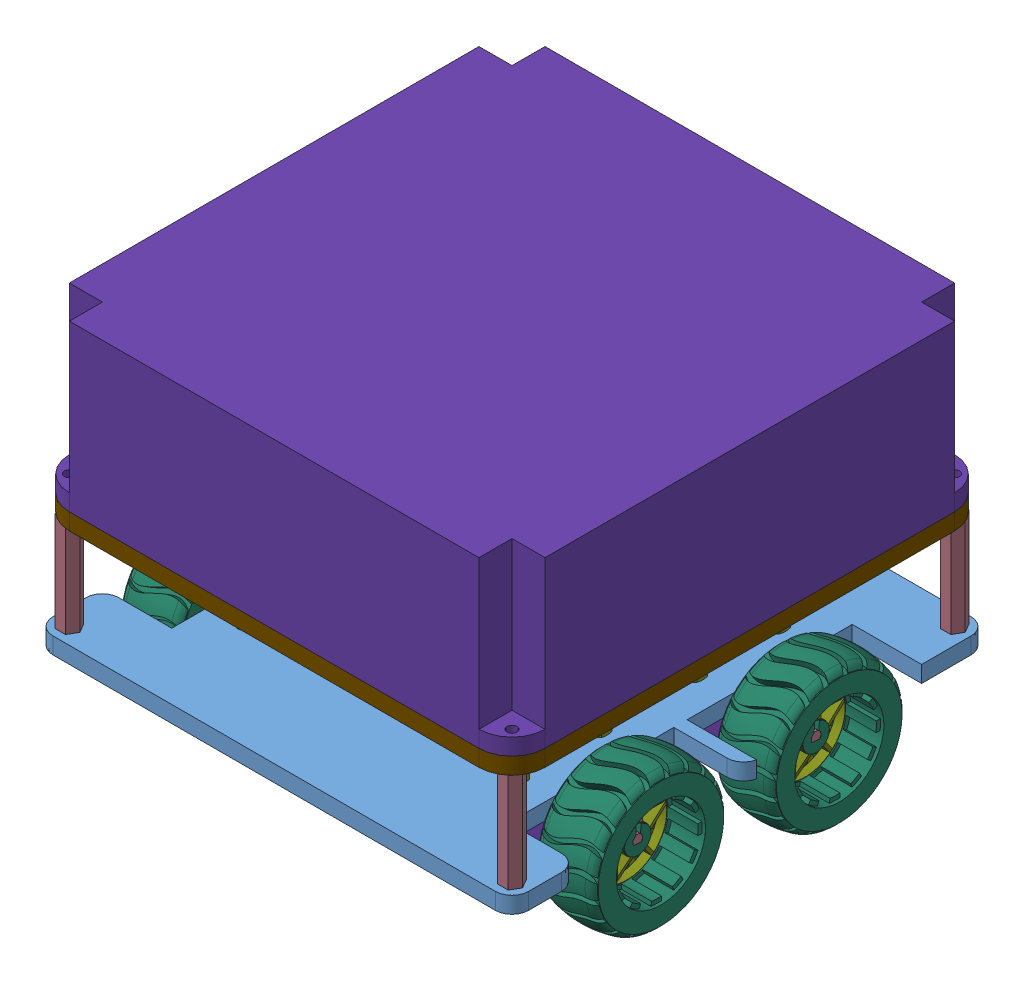
SolidWorks assembly 4 WHEELED BOT, configuration Default. Lengths in mm.
Overall size (144.48 119.43 144).
160 component instances, 35 part files, 86 mates.
Components (placement in the parent):
- BASE-1: BASE [Default] at (33.0776 85.5576 114.3688) size (144 5 144)
- Motor complete assembly-1: Motor complete assembly [Default] at (60.6046 55.5446 163.4077) x (1 0 0) z (0 1 0) size (47.72 49.6 49.13)
  - MOTOR ASSEMBLY-1: MOTOR ASSEMBLY [По умолчанию] at (3.7017 9.4456 12.6365) size (40.48 13.3 19.35)
    - H-1: H [По умолчанию] at (2.1713 12.5934 12.3765) size (17.5 12.02 10)
    - spur gear_iso-1: spur gear_iso [ISO - Spur gear 0.25M 11T 20PA 1.5FW ---S11A75H50L1.0N] at (15.9213 12.5934 12.3765) x (1 0 0) z (0 0.090891 -0.995861) size (1.5 3.2 3.23)
    - I-1: I [По умолчанию] at (14.6713 12.5934 12.3765) x (0 1 0) z (1 0 0) size (12 10 0.8)
    - G-1: G [По умолчанию] at (17.9713 16.1934 15.3765) x (0 0 1) z (0 -1 0) size (3 2.5 3)
    - G-2: G [По умолчанию] at (15.4713 8.9934 9.3765) x (0 1 0) z (0 0 -1) size (3 2.5 3)
    - J-1: J [По умолчанию] at (17.9713 12.5934 12.3765) x (0 -1 0) z (1 0 0) size (12 10 0.8)
    - A-1: A [По умолчанию] at (22.9713 16.1934 15.3765) x (0 -0.998437 -0.055897) z (0 0.055897 -0.998437) size (3 4.2 3)
    - A-2: A [По умолчанию] at (18.7713 8.9934 9.3765) x (0 0.267458 -0.96357) z (0 -0.96357 -0.267458) size (3 4.2 3)
    - C-1: C [По умолчанию] at (22.9713 12.5934 12.3765) x (0 1 0) z (1 0 0) size (12 10 1.8)
    - spur gear_iso-2: spur gear_iso [ISO - Spur gear 0.25M 20T 20PA 1,5FW ---S20B6H1,7L0.8N] at (17.9713 12.5934 12.3765) x (-1 0 0) z (0 0.996827 -0.079597) size (1.7 5.45 5.45)
    - F-1: F [По умолчанию] at (17.9713 9.3434 14.3765) x (0 0.378034 -0.925792) z (0 -0.925792 -0.378034) size (0.75 5.8 0.75)
    - E-1: E [По умолчанию] at (17.9713 12.5934 12.3765) x (0 0.298251 0.954488) z (0 0.954488 -0.298251) size (0.75 3.5 0.75)
    - spur gear_iso-3: spur gear_iso [ISO - Spur gear 0.25M 20T 20PA 1FW ---S20A75H50L0.8N] at (18.8713 12.5934 12.3765) x (1 0 0) z (0 0.821933 -0.569584) size (1 5.45 5.45)
    - spur gear_iso-4: spur gear_iso [ISO - Spur gear 0.25M 10T 20PA 1,3FW ---S10A75H50L0.8N] at (19.8713 12.5934 12.3765) x (1 0 0) z (0 -0.579316 0.815103) size (1.3 2.87 3)
    - spur gear_iso-6: spur gear_iso [ISO - Spur gear 0.25M 10T 20PA 1,7FW ---S10A75H50L0.8N] at (16.3713 9.3434 14.3765) x (1 0 0) z (0 -0.299679 -0.95404) size (1.7 2.87 3)
    - spur gear_iso-7: spur gear_iso [ISO - Spur gear 0.25M 20T 20PA 1,2FW ---S20A75H50L0.8N] at (19.9713 9.3434 14.3765) x (1 0 0) z (0 0.932152 0.362067) size (1.2 5.45 5.45)
    - D-1: D [По умолчанию] at (14.6713 15.8434 10.3765) x (0 0 -1) z (0 -1 0) size (0.75 9.1 0.75)
    - spur gear_iso-8: spur gear_iso [ISO - Spur gear 0.25M 20T 20PA 1,5FW ---S20A75H50L0.8N] at (15.9213 15.8434 10.3765) x (1 0 0) z (0 -0.974451 0.2246) size (1.5 5.45 5.45)
    - spur gear_iso-9: spur gear_iso [ISO - Spur gear 0.25M 10T 20PA 3,5FW ---S10A75H50L0.8N] at (17.4213 15.8434 10.3765) x (1 0 0) z (0 0.96714 0.254244) size (3.5 2.87 3)
    - motor back part-1: motor back part [Default] at (1.1713 12.5934 12.3765) x (0 0 1) z (-1 0 0) size (10 11.89 1.02)
    - B-2: B [По умолчанию] at (22.9713 12.5934 12.3765) x (0 0.071836 0.997416) z (0 0.997416 -0.071836) size (3 12.3 3)
    - K-2: K [Default] at (0.1713 12.5934 12.3765) x (0 -0.999909 0.013511) z (-1 0 0) size (12 19 7.88)
  - RC wheel-1: RC wheel [Default] at (14.1964 -16.5261 -2.5515) x (0 0.997416 -0.071836) z (1 0 0) size (46.42 45.91 18.48)
    - Housing-1: Housing [Default] at (36.5766 30.151 12.2766) size (46.42 45.91 18.48)
    - Hub-1: Hub [Default] at (36.5766 30.151 17.1766) x (-0.261271 -0.965266 0) z (-0.965266 0.261271 0) size (24.5 5.75 24.5)
  - gear motor clamp-1: gear motor clamp [Default] at (18.373 22.0389 30.013) x (0 1 0) z (-1 0 0) size (36 13 11)
- Motor complete assembly-2: Motor complete assembly [Default] at (60.6046 55.5446 109.4077) x (1 0 0) z (0 1 0) size (47.72 49.6 49.13)
  - MOTOR ASSEMBLY-1: MOTOR ASSEMBLY [По умолчанию] at (3.7017 9.4456 12.6365) size (40.48 13.3 19.35)
    - H-1: H [По умолчанию] at (2.1713 12.5934 12.3765) size (17.5 12.02 10)
    - spur gear_iso-1: spur gear_iso [ISO - Spur gear 0.25M 11T 20PA 1.5FW ---S11A75H50L1.0N] at (15.9213 12.5934 12.3765) x (1 0 0) z (0 0.090891 -0.995861) size (1.5 3.2 3.23)
    - I-1: I [По умолчанию] at (14.6713 12.5934 12.3765) x (0 1 0) z (1 0 0) size (12 10 0.8)
    - G-1: G [По умолчанию] at (17.9713 16.1934 15.3765) x (0 0 1) z (0 -1 0) size (3 2.5 3)
    - G-2: G [По умолчанию] at (15.4713 8.9934 9.3765) x (0 1 0) z (0 0 -1) size (3 2.5 3)
    - J-1: J [По умолчанию] at (17.9713 12.5934 12.3765) x (0 -1 0) z (1 0 0) size (12 10 0.8)
    - A-1: A [По умолчанию] at (22.9713 16.1934 15.3765) x (0 -0.998437 -0.055897) z (0 0.055897 -0.998437) size (3 4.2 3)
    - A-2: A [По умолчанию] at (18.7713 8.9934 9.3765) x (0 0.267458 -0.96357) z (0 -0.96357 -0.267458) size (3 4.2 3)
    - C-1: C [По умолчанию] at (22.9713 12.5934 12.3765) x (0 1 0) z (1 0 0) size (12 10 1.8)
    - spur gear_iso-2: spur gear_iso [ISO - Spur gear 0.25M 20T 20PA 1,5FW ---S20B6H1,7L0.8N] at (17.9713 12.5934 12.3765) x (-1 0 0) z (0 0.996827 -0.079597) size (1.7 5.45 5.45)
    - F-1: F [По умолчанию] at (17.9713 9.3434 14.3765) x (0 0.378034 -0.925792) z (0 -0.925792 -0.378034) size (0.75 5.8 0.75)
    - E-1: E [По умолчанию] at (17.9713 12.5934 12.3765) x (0 0.298251 0.954488) z (0 0.954488 -0.298251) size (0.75 3.5 0.75)
    - spur gear_iso-3: spur gear_iso [ISO - Spur gear 0.25M 20T 20PA 1FW ---S20A75H50L0.8N] at (18.8713 12.5934 12.3765) x (1 0 0) z (0 0.821933 -0.569584) size (1 5.45 5.45)
    - spur gear_iso-4: spur gear_iso [ISO - Spur gear 0.25M 10T 20PA 1,3FW ---S10A75H50L0.8N] at (19.8713 12.5934 12.3765) x (1 0 0) z (0 -0.579316 0.815103) size (1.3 2.87 3)
    - spur gear_iso-6: spur gear_iso [ISO - Spur gear 0.25M 10T 20PA 1,7FW ---S10A75H50L0.8N] at (16.3713 9.3434 14.3765) x (1 0 0) z (0 -0.299679 -0.95404) size (1.7 2.87 3)
    - spur gear_iso-7: spur gear_iso [ISO - Spur gear 0.25M 20T 20PA 1,2FW ---S20A75H50L0.8N] at (19.9713 9.3434 14.3765) x (1 0 0) z (0 0.932152 0.362067) size (1.2 5.45 5.45)
    - D-1: D [По умолчанию] at (14.6713 15.8434 10.3765) x (0 0 -1) z (0 -1 0) size (0.75 9.1 0.75)
    - spur gear_iso-8: spur gear_iso [ISO - Spur gear 0.25M 20T 20PA 1,5FW ---S20A75H50L0.8N] at (15.9213 15.8434 10.3765) x (1 0 0) z (0 -0.974451 0.2246) size (1.5 5.45 5.45)
    - spur gear_iso-9: spur gear_iso [ISO - Spur gear 0.25M 10T 20PA 3,5FW ---S10A75H50L0.8N] at (17.4213 15.8434 10.3765) x (1 0 0) z (0 0.96714 0.254244) size (3.5 2.87 3)
    - motor back part-1: motor back part [Default] at (1.1713 12.5934 12.3765) x (0 0 1) z (-1 0 0) size (10 11.89 1.02)
    - B-2: B [По умолчанию] at (22.9713 12.5934 12.3765) x (0 0.071836 0.997416) z (0 0.997416 -0.071836) size (3 12.3 3)
    - K-2: K [Default] at (0.1713 12.5934 12.3765) x (0 -0.999909 0.013511) z (-1 0 0) size (12 19 7.88)
  - RC wheel-1: RC wheel [Default] at (14.1964 -16.5261 -2.5515) x (0 0.997416 -0.071836) z (1 0 0) size (46.42 45.91 18.48)
    - Housing-1: Housing [Default] at (36.5766 30.151 12.2766) size (46.42 45.91 18.48)
    - Hub-1: Hub [Default] at (36.5766 30.151 17.1766) x (-0.261271 -0.965266 0) z (-0.965266 0.261271 0) size (24.5 5.75 24.5)
  - gear motor clamp-1: gear motor clamp [Default] at (18.373 22.0389 30.013) x (0 1 0) z (-1 0 0) size (36 13 11)
- Motor complete assembly-3: Motor complete assembly [Default] at (5.5507 55.5446 65.3299) x (-1 0 0) z (0 1 0) size (47.72 49.6 49.13)
  - MOTOR ASSEMBLY-1: MOTOR ASSEMBLY [По умолчанию] at (3.7017 9.4456 12.6365) size (40.48 13.3 19.35)
    - H-1: H [По умолчанию] at (2.1713 12.5934 12.3765) size (17.5 12.02 10)
    - spur gear_iso-1: spur gear_iso [ISO - Spur gear 0.25M 11T 20PA 1.5FW ---S11A75H50L1.0N] at (15.9213 12.5934 12.3765) x (1 0 0) z (0 0.090891 -0.995861) size (1.5 3.2 3.23)
    - I-1: I [По умолчанию] at (14.6713 12.5934 12.3765) x (0 1 0) z (1 0 0) size (12 10 0.8)
    - G-1: G [По умолчанию] at (17.9713 16.1934 15.3765) x (0 0 1) z (0 -1 0) size (3 2.5 3)
    - G-2: G [По умолчанию] at (15.4713 8.9934 9.3765) x (0 1 0) z (0 0 -1) size (3 2.5 3)
    - J-1: J [По умолчанию] at (17.9713 12.5934 12.3765) x (0 -1 0) z (1 0 0) size (12 10 0.8)
    - A-1: A [По умолчанию] at (22.9713 16.1934 15.3765) x (0 -0.998437 -0.055897) z (0 0.055897 -0.998437) size (3 4.2 3)
    - A-2: A [По умолчанию] at (18.7713 8.9934 9.3765) x (0 0.267458 -0.96357) z (0 -0.96357 -0.267458) size (3 4.2 3)
    - C-1: C [По умолчанию] at (22.9713 12.5934 12.3765) x (0 1 0) z (1 0 0) size (12 10 1.8)
    - spur gear_iso-2: spur gear_iso [ISO - Spur gear 0.25M 20T 20PA 1,5FW ---S20B6H1,7L0.8N] at (17.9713 12.5934 12.3765) x (-1 0 0) z (0 0.996827 -0.079597) size (1.7 5.45 5.45)
    - F-1: F [По умолчанию] at (17.9713 9.3434 14.3765) x (0 0.378034 -0.925792) z (0 -0.925792 -0.378034) size (0.75 5.8 0.75)
    - E-1: E [По умолчанию] at (17.9713 12.5934 12.3765) x (0 0.298251 0.954488) z (0 0.954488 -0.298251) size (0.75 3.5 0.75)
    - spur gear_iso-3: spur gear_iso [ISO - Spur gear 0.25M 20T 20PA 1FW ---S20A75H50L0.8N] at (18.8713 12.5934 12.3765) x (1 0 0) z (0 0.821933 -0.569584) size (1 5.45 5.45)
    - spur gear_iso-4: spur gear_iso [ISO - Spur gear 0.25M 10T 20PA 1,3FW ---S10A75H50L0.8N] at (19.8713 12.5934 12.3765) x (1 0 0) z (0 -0.579316 0.815103) size (1.3 2.87 3)
    - spur gear_iso-6: spur gear_iso [ISO - Spur gear 0.25M 10T 20PA 1,7FW ---S10A75H50L0.8N] at (16.3713 9.3434 14.3765) x (1 0 0) z (0 -0.299679 -0.95404) size (1.7 2.87 3)
    - spur gear_iso-7: spur gear_iso [ISO - Spur gear 0.25M 20T 20PA 1,2FW ---S20A75H50L0.8N] at (19.9713 9.3434 14.3765) x (1 0 0) z (0 0.932152 0.362067) size (1.2 5.45 5.45)
    - D-1: D [По умолчанию] at (14.6713 15.8434 10.3765) x (0 0 -1) z (0 -1 0) size (0.75 9.1 0.75)
    - spur gear_iso-8: spur gear_iso [ISO - Spur gear 0.25M 20T 20PA 1,5FW ---S20A75H50L0.8N] at (15.9213 15.8434 10.3765) x (1 0 0) z (0 -0.974451 0.2246) size (1.5 5.45 5.45)
    - spur gear_iso-9: spur gear_iso [ISO - Spur gear 0.25M 10T 20PA 3,5FW ---S10A75H50L0.8N] at (17.4213 15.8434 10.3765) x (1 0 0) z (0 0.96714 0.254244) size (3.5 2.87 3)
    - motor back part-1: motor back part [Default] at (1.1713 12.5934 12.3765) x (0 0 1) z (-1 0 0) size (10 11.89 1.02)
    - B-2: B [По умолчанию] at (22.9713 12.5934 12.3765) x (0 0.071836 0.997416) z (0 0.997416 -0.071836) size (3 12.3 3)
    - K-2: K [Default] at (0.1713 12.5934 12.3765) x (0 -0.999909 0.013511) z (-1 0 0) size (12 19 7.88)
  - RC wheel-1: RC wheel [Default] at (14.1964 -16.5261 -2.5515) x (0 0.997416 -0.071836) z (1 0 0) size (46.42 45.91 18.48)
    - Housing-1: Housing [Default] at (36.5766 30.151 12.2766) size (46.42 45.91 18.48)
    - Hub-1: Hub [Default] at (36.5766 30.151 17.1766) x (-0.261271 -0.965266 0) z (-0.965266 0.261271 0) size (24.5 5.75 24.5)
  - gear motor clamp-1: gear motor clamp [Default] at (18.373 22.0389 30.013) x (0 1 0) z (-1 0 0) size (36 13 11)
- Motor complete assembly-4: Motor complete assembly [Default] at (5.5507 55.5446 119.3299) x (-1 0 0) z (0 1 0) size (47.72 49.6 49.13)
  - MOTOR ASSEMBLY-1: MOTOR ASSEMBLY [По умолчанию] at (3.7017 9.4456 12.6365) size (40.48 13.3 19.35)
    - H-1: H [По умолчанию] at (2.1713 12.5934 12.3765) size (17.5 12.02 10)
    - spur gear_iso-1: spur gear_iso [ISO - Spur gear 0.25M 11T 20PA 1.5FW ---S11A75H50L1.0N] at (15.9213 12.5934 12.3765) x (1 0 0) z (0 0.090891 -0.995861) size (1.5 3.2 3.23)
    - I-1: I [По умолчанию] at (14.6713 12.5934 12.3765) x (0 1 0) z (1 0 0) size (12 10 0.8)
    - G-1: G [По умолчанию] at (17.9713 16.1934 15.3765) x (0 0 1) z (0 -1 0) size (3 2.5 3)
    - G-2: G [По умолчанию] at (15.4713 8.9934 9.3765) x (0 1 0) z (0 0 -1) size (3 2.5 3)
    - J-1: J [По умолчанию] at (17.9713 12.5934 12.3765) x (0 -1 0) z (1 0 0) size (12 10 0.8)
    - A-1: A [По умолчанию] at (22.9713 16.1934 15.3765) x (0 -0.998437 -0.055897) z (0 0.055897 -0.998437) size (3 4.2 3)
    - A-2: A [По умолчанию] at (18.7713 8.9934 9.3765) x (0 0.267458 -0.96357) z (0 -0.96357 -0.267458) size (3 4.2 3)
    - C-1: C [По умолчанию] at (22.9713 12.5934 12.3765) x (0 1 0) z (1 0 0) size (12 10 1.8)
    - spur gear_iso-2: spur gear_iso [ISO - Spur gear 0.25M 20T 20PA 1,5FW ---S20B6H1,7L0.8N] at (17.9713 12.5934 12.3765) x (-1 0 0) z (0 0.996827 -0.079597) size (1.7 5.45 5.45)
    - F-1: F [По умолчанию] at (17.9713 9.3434 14.3765) x (0 0.378034 -0.925792) z (0 -0.925792 -0.378034) size (0.75 5.8 0.75)
    - E-1: E [По умолчанию] at (17.9713 12.5934 12.3765) x (0 0.298251 0.954488) z (0 0.954488 -0.298251) size (0.75 3.5 0.75)
    - spur gear_iso-3: spur gear_iso [ISO - Spur gear 0.25M 20T 20PA 1FW ---S20A75H50L0.8N] at (18.8713 12.5934 12.3765) x (1 0 0) z (0 0.821933 -0.569584) size (1 5.45 5.45)
    - spur gear_iso-4: spur gear_iso [ISO - Spur gear 0.25M 10T 20PA 1,3FW ---S10A75H50L0.8N] at (19.8713 12.5934 12.3765) x (1 0 0) z (0 -0.579316 0.815103) size (1.3 2.87 3)
    - spur gear_iso-6: spur gear_iso [ISO - Spur gear 0.25M 10T 20PA 1,7FW ---S10A75H50L0.8N] at (16.3713 9.3434 14.3765) x (1 0 0) z (0 -0.299679 -0.95404) size (1.7 2.87 3)
    - spur gear_iso-7: spur gear_iso [ISO - Spur gear 0.25M 20T 20PA 1,2FW ---S20A75H50L0.8N] at (19.9713 9.3434 14.3765) x (1 0 0) z (0 0.932152 0.362067) size (1.2 5.45 5.45)
    - D-1: D [По умолчанию] at (14.6713 15.8434 10.3765) x (0 0 -1) z (0 -1 0) size (0.75 9.1 0.75)
    - spur gear_iso-8: spur gear_iso [ISO - Spur gear 0.25M 20T 20PA 1,5FW ---S20A75H50L0.8N] at (15.9213 15.8434 10.3765) x (1 0 0) z (0 -0.974451 0.2246) size (1.5 5.45 5.45)
    - spur gear_iso-9: spur gear_iso [ISO - Spur gear 0.25M 10T 20PA 3,5FW ---S10A75H50L0.8N] at (17.4213 15.8434 10.3765) x (1 0 0) z (0 0.96714 0.254244) size (3.5 2.87 3)
    - motor back part-1: motor back part [Default] at (1.1713 12.5934 12.3765) x (0 0 1) z (-1 0 0) size (10 11.89 1.02)
    - B-2: B [По умолчанию] at (22.9713 12.5934 12.3765) x (0 0.071836 0.997416) z (0 0.997416 -0.071836) size (3 12.3 3)
    - K-2: K [Default] at (0.1713 12.5934 12.3765) x (0 -0.999909 0.013511) z (-1 0 0) size (12 19 7.88)
  - RC wheel-1: RC wheel [Default] at (14.1964 -16.5261 -2.5515) x (0 0.997416 -0.071836) z (1 0 0) size (46.42 45.91 18.48)
    - Housing-1: Housing [Default] at (36.5766 30.151 12.2766) size (46.42 45.91 18.48)
    - Hub-1: Hub [Default] at (36.5766 30.151 17.1766) x (-0.261271 -0.965266 0) z (-0.965266 0.261271 0) size (24.5 5.75 24.5)
  - gear motor clamp-1: gear motor clamp [Default] at (18.373 22.0389 30.013) x (0 1 0) z (-1 0 0) size (36 13 11)
- middle compartment-1: middle compartment [Default] at (33.0776 120.5576 114.3688) size (144 5 144)
- Servo with clamp v2-1: Servo with clamp v2 [Default] at (72.9153 150.9247 62.9785) x (0 0 1) z (0 -1 0) size (92 44.85 25)
  - mg995 servo-1: mg995 servo [Predeterminado] at (24.2303 26.1277 40.4571) size (53.82 44.84 19.95)
  - SERVO CLAMP-1: SERVO CLAMP [Default] at (25.3903 36.3177 30.3671) x (1 0 0) z (0 -1 0) size (92 25 15)
- cube-1: cube [Default] at (21.6376 98.5576 47.3688) size (20 20 20)
- LM2596 Buck Converter 4.0-40 to 1.3-37V-1: LM2596 Buck Converter 4.0-40 to 1.3-37V [Default] at (57.0776 135.5576 153.3688) size (66 17.65 36)
  - BASE,  LM2596 Buck Converter 4.0-40 to 1.3-37V-1: BASE,  LM2596 Buck Converter 4.0-40 to 1.3-37V [Default] at origin size (66 1.6 36)
  - DG301-5.0-02, LM2596 Buck Converter 4.0-40 to 1.3-37V-3: DG301-5.0-02, LM2596 Buck Converter 4.0-40 to 1.3-37V [Default] at (29.9 1.6 2.5) x (0 0 -1) z (0 1 0) size (10.6 7.6 14.3)
  - DG301-5.0-02, LM2596 Buck Converter 4.0-40 to 1.3-37V-2: DG301-5.0-02, LM2596 Buck Converter 4.0-40 to 1.3-37V [Default] at (-29.9 1.6 -2.5) x (0 0 1) z (0 1 0) size (10.6 7.6 14.3)
  - 3 DIGIT 7 SEGMENT DISPLAY, LM2596 Buck Converter 4.0-40 to 1.3-37V-1: 3 DIGIT 7 SEGMENT DISPLAY, LM2596 Buck Converter 4.0-40 to 1.3-37V [Default] at (0 8.8 11) size (22.5 13.3 14)
  - Trimpot 3296W, LM2596 Buck Converter 4.0-40 to 1.3-37V-1: Trimpot 3296W, LM2596 Buck Converter 4.0-40 to 1.3-37V [Valor predeterminado] at (5.235 1.6 -15.585) x (-1 0 0) z (0 1 0) size (9.53 4.83 14.15)
  - 220 35V CAPACITOR, LM2596 Buck Converter 4.0-40 to 1.3-37V-1: 220 35V CAPACITOR, LM2596 Buck Converter 4.0-40 to 1.3-37V [Default] at (-19.85 1.6 -7.85) size (8.3 10.5 8.3)
  - 220 35V CAPACITOR, LM2596 Buck Converter 4.0-40 to 1.3-37V-2: 220 35V CAPACITOR, LM2596 Buck Converter 4.0-40 to 1.3-37V [Default] at (18.25 1.6 -6.85) size (8.3 10.5 8.3)
- ESP 32-1: ESP 32 [Default] at (35.9526 130.1576 83.6258) x (-1 0 0) z (0 0 1) size (25.91 13.14 49.31)
- L298N 12-48V 2A 2 moteurs-1: L298N 12-48V 2A 2 moteurs [Défaut] at (73.4526 130.5576 78.9688) x (1 0 0) z (0 1 0) size (43.25 43.26 26.16)
- Battery outline-1: Battery outline [Default] at (3.0776 125.5576 114.3688) x (0 0 -1) z (1 0 0) size (106 23 34)
- battery clamp-1: battery clamp [Default] at (3.0776 123.5576 114.3688) size (74 30 15)
- M3 30MM F-F-1: M3 30MM F-F [Default] at (-33.9224 90.5576 47.3688) x (-0.837169 0 -0.546944) z (0 1 0) size (6.35 5.5 30)
- M3 30MM F-F-2: M3 30MM F-F [Default] at (100.0776 90.5576 47.3688) x (1 0 0) z (0 1 0) size (6.35 5.5 30)
- M3 30MM F-F-3: M3 30MM F-F [Default] at (100.0776 90.5576 181.3688) x (1 0 0) z (0 1 0) size (6.35 5.5 30)
- M3 30MM F-F-4: M3 30MM F-F [Default] at (-33.9224 120.5576 181.3688) x (1 0 0) z (0 -1 0) size (6.35 5.5 30)
- TOWER PRO MG-995, ANALOG SERVO, HORN-1: TOWER PRO MG-995, ANALOG SERVO, HORN [Default] at (23.2376 110.4676 76.9588) x (0 0.078015 -0.996952) z (0 0.996952 0.078015) size (12.7 5.75 24.43)
- pan slot head_am-1: pan slot head_am [B18.6.7M - M3 x 0.5 x 13 Slotted PHMS --13N] at (73.4776 80.1576 153.8688) x (0 1 0) z (0 0 1) size (15.48 5.6 5.6)
- pan slot head_am-2: pan slot head_am [B18.6.7M - M3 x 0.5 x 13 Slotted PHMS --13N] at (73.4776 80.1576 128.8688) x (0 1 0) z (0 0 1) size (15.48 5.6 5.6)
- pan slot head_am-3: pan slot head_am [B18.6.7M - M3 x 0.5 x 13 Slotted PHMS --13N] at (73.4776 80.1576 99.8688) x (0 1 0) z (0 0 1) size (15.48 5.6 5.6)
- pan slot head_am-4: pan slot head_am [B18.6.7M - M3 x 0.5 x 13 Slotted PHMS --13N] at (73.4776 80.1576 74.8688) x (0 1 0) z (0 0 1) size (15.48 5.6 5.6)
- pan slot head_am-5: pan slot head_am [B18.6.7M - M3 x 0.5 x 13 Slotted PHMS --13N] at (-7.3224 80.1576 74.8688) x (0 1 0) z (0 0 1) size (15.48 5.6 5.6)
- pan slot head_am-6: pan slot head_am [B18.6.7M - M3 x 0.5 x 13 Slotted PHMS --13N] at (-7.3224 80.1576 99.8688) x (0 1 0) z (0 0 1) size (15.48 5.6 5.6)
- pan slot head_am-7: pan slot head_am [B18.6.7M - M3 x 0.5 x 13 Slotted PHMS --13N] at (-7.3224 80.1576 128.8688) x (0 1 0) z (0 0 1) size (15.48 5.6 5.6)
- pan slot head_am-8: pan slot head_am [B18.6.7M - M3 x 0.5 x 13 Slotted PHMS --13N] at (-7.3224 80.1576 153.8688) x (0 1 0) z (0 0 1) size (15.48 5.6 5.6)
- pan slot head_am-9: pan slot head_am [B18.6.7M - M3 x 0.5 x 13 Slotted PHMS --13N] at (-25.1724 128.9576 121.8688) x (0 -1 0) z (0 0 1) size (15.48 5.6 5.6)
- pan slot head_am-10: pan slot head_am [B18.6.7M - M3 x 0.5 x 13 Slotted PHMS --13N] at (31.3276 128.9576 121.8688) x (0 -1 0) z (0 0 1) size (15.48 5.6 5.6)
- pan slot head_am-11: pan slot head_am [B18.6.7M - M3 x 0.5 x 13 Slotted PHMS --13N] at (44.0976 113.1576 53.6188) x (0 1 0) z (0 0 1) size (15.48 5.6 5.6)
- pan slot head_am-12: pan slot head_am [B18.6.7M - M3 x 0.5 x 13 Slotted PHMS --13N] at (44.0976 113.1576 123.1188) x (0 1 0) z (0 0 1) size (15.48 5.6 5.6)
- hex nut style 2_am-1: hex nut style 2_am [B18.2.4.2M - Hex nut, Style 2,  M3 x 0.5 --D-N] at (-25.1724 119.8276 121.8688) x (1 0 0) z (0 1 0) size (5.5 6.35 2.9)
- hex nut style 2_am-3: hex nut style 2_am [B18.2.4.2M - Hex nut, Style 2,  M3 x 0.5 --D-N] at (31.3276 119.8182 121.8688) x (1 0 0) z (0 1 0) size (5.5 6.35 2.9)
- hex nut style 2_am-4: hex nut style 2_am [B18.2.4.2M - Hex nut, Style 2,  M3 x 0.5 --D-N] at (44.0976 125.5534 53.6188) x (1 0 0) z (0 -1 0) size (5.5 6.35 2.9)
- hex nut style 2_am-5: hex nut style 2_am [B18.2.4.2M - Hex nut, Style 2,  M3 x 0.5 --D-N] at (73.4776 90.7212 153.8688) x (1 0 0) z (0 -1 0) size (5.5 6.35 2.9)
- hex nut style 2_am-6: hex nut style 2_am [B18.2.4.2M - Hex nut, Style 2,  M3 x 0.5 --D-N] at (73.4776 90.7695 128.8688) x (1 0 0) z (0 -1 0) size (5.5 6.35 2.9)
- hex nut style 2_am-7: hex nut style 2_am [B18.2.4.2M - Hex nut, Style 2,  M3 x 0.5 --D-N] at (73.4776 90.7674 99.8688) x (1 0 0) z (0 -1 0) size (5.5 6.35 2.9)
- hex nut style 2_am-8: hex nut style 2_am [B18.2.4.2M - Hex nut, Style 2,  M3 x 0.5 --D-N] at (73.4776 90.9568 74.8688) x (1 0 0) z (0 -1 0) size (5.5 6.35 2.9)
- hex nut style 2_am-9: hex nut style 2_am [B18.2.4.2M - Hex nut, Style 2,  M3 x 0.5 --D-N] at (-7.3224 90.7611 153.8688) x (1 0 0) z (0 -1 0) size (5.5 6.35 2.9)
- hex nut style 2_am-10: hex nut style 2_am [B18.2.4.2M - Hex nut, Style 2,  M3 x 0.5 --D-N] at (-7.3224 90.826 128.8688) x (1 0 0) z (0 -1 0) size (5.5 6.35 2.9)
- hex nut style 2_am-11: hex nut style 2_am [B18.2.4.2M - Hex nut, Style 2,  M3 x 0.5 --D-N] at (-7.3224 90.6697 99.8688) x (1 0 0) z (0 -1 0) size (5.5 6.35 2.9)
- hex nut style 2_am-15: hex nut style 2_am [B18.2.4.2M - Hex nut, Style 2,  M3 x 0.5 --D-N] at (44.0976 128.4576 123.1188) x (1 0 0) z (0 1 0) size (5.5 6.35 2.9)
- hex nut style 2_am-17: hex nut style 2_am [B18.2.4.2M - Hex nut, Style 2,  M3 x 0.5 --D-N] at (-7.3224 91.1226 74.8688) x (1 0 0) z (0 -1 0) size (5.5 6.35 2.9)
- ENCLOSURE-1: ENCLOSURE [Default] at (33.0776 125.5576 114.3688) size (144 50 144)
Mates (geometry in assembly coordinates):
- Coincident17: coincident aligned: plane of BASE-1 through (105.0776 90.5576 42.3688) normal (1 0 0); plane of Motor complete assembly-2/RC wheel-1/Housing-1 through (105.0776 80.4387 87.2858) normal (1 0 0)
- Width1: width aligned: plane of BASE-1 through (84.0776 85.5576 112.3688) normal (0 0 -1); plane of BASE-1 through (105.0776 85.5576 62.3688) normal (0 0 1); plane of Motor complete assembly-2/gear motor clamp-1 through (67.9776 82.5576 78.3688) normal (0 0 -1); plane of Motor complete assembly-2/gear motor clamp-1 through (67.9776 82.5576 96.3688) normal (0 0 1)
- Width2: width aligned: plane of BASE-1 through (105.0776 85.5576 166.3688) normal (0 0 -1); plane of BASE-1 through (84.0776 85.5576 116.3688) normal (0 0 1); plane of Motor complete assembly-1/gear motor clamp-1 through (67.9776 82.5576 132.3688) normal (0 0 -1); plane of Motor complete assembly-1/gear motor clamp-1 through (67.9776 82.5576 150.3688) normal (0 0 1)
- Coincident20: coincident aligned: plane of BASE-1 through (105.0776 90.5576 42.3688) normal (1 0 0); plane of Motor complete assembly-1/RC wheel-1/Housing-1 through (105.0776 80.4387 141.2858) normal (1 0 0)
- Width3: width anti-aligned: plane of BASE-1 through (-17.9224 85.5576 116.3688) normal (0 0 1); plane of BASE-1 through (-38.9224 85.5576 166.3688) normal (0 0 -1); plane of Motor complete assembly-4/gear motor clamp-1 through (-1.8224 82.5576 132.3688) normal (0 0 -1); plane of Motor complete assembly-4/gear motor clamp-1 through (-1.8224 82.5576 150.3688) normal (0 0 1)
- Coincident21: coincident aligned: plane of BASE-1 through (-38.9224 90.5576 42.3688) normal (-1 0 0); plane of Motor complete assembly-4/RC wheel-1/Housing-1 through (-38.9224 80.4387 141.4518) normal (-1 0 0)
- Width4: width aligned: plane of BASE-1 through (-38.9224 85.5576 62.3688) normal (0 0 1); plane of BASE-1 through (-17.9224 85.5576 112.3688) normal (0 0 -1); plane of Motor complete assembly-3/gear motor clamp-1 through (-1.8224 82.5576 96.3688) normal (0 0 1); plane of Motor complete assembly-3/gear motor clamp-1 through (-1.8224 82.5576 78.3688) normal (0 0 -1)
- Coincident22: coincident aligned: plane of BASE-1 through (-38.9224 90.5576 42.3688) normal (-1 0 0); plane of Motor complete assembly-3/RC wheel-1/Housing-1 through (-38.9224 80.4387 87.4518) normal (-1 0 0)
- Distance1: distance = 30 mm anti-aligned: plane of BASE-1 through (33.0776 90.5576 114.3688) normal (0 1 0); plane of middle compartment-1 through (33.0776 120.5576 114.3688) normal (0 -1 0)
- Coincident24: coincident aligned: plane of BASE-1 through (-38.9224 90.5576 42.3688) normal (0 0 -1); plane of middle compartment-1 through (-38.9224 125.5576 42.3688) normal (0 0 -1)
- Coincident25: coincident aligned: plane of BASE-1 through (-38.9224 90.5576 42.3688) normal (-1 0 0); plane of middle compartment-1 through (-38.9224 125.5576 42.3688) normal (-1 0 0)
- Coincident26: coincident anti-aligned: plane of middle compartment-1 through (33.0776 120.5576 114.3688) normal (0 -1 0); plane of Servo with clamp v2-1/SERVO CLAMP-1 through (51.5976 120.5576 68.3688) normal (0 1 0)
- Coincident27: coincident aligned: plane of middle compartment-1 through (-38.9224 125.5576 42.3688) normal (0 0 -1); plane of Servo with clamp v2-1/SERVO CLAMP-1 through (51.5976 120.5576 42.3688) normal (0 0 -1)
- Distance2: distance = 40 mm aligned: plane of middle compartment-1 through (105.0776 125.5576 42.3688) normal (1 0 0); plane of Servo with clamp v2-1/mg995 servo-1 through (65.0776 100.5576 67.0488) normal (1 0 0)
- Coincident29: coincident anti-aligned: plane of BASE-1 through (33.0776 88.5576 114.3688) normal (0 1 0); plane of cube-1 through (11.6376 88.5576 67.3688) normal (0 -1 0)
- Distance19: distance = 5 mm aligned: plane of BASE-1 through (-38.9224 90.5576 42.3688) normal (0 0 -1); plane of cube-1 through (21.6376 98.5576 47.3688) normal (0 0 -1)
- Distance3: distance = 1 mm anti-aligned: plane of cube-1 through (11.6376 108.5576 67.3688) normal (-1 0 0); plane of BASE-1 through (10.6376 88.5576 42.3688) normal (1 0 0)
- Distance7: distance = 10 mm anti-aligned: plane of middle compartment-1 through (33.0776 125.5576 114.3688) normal (0 1 0); plane of LM2596 Buck Converter 4.0-40 to 1.3-37V-1/BASE,  LM2596 Buck Converter 4.0-40 to 1.3-37V-1 through (57.0776 135.5576 153.3688) normal (0 -1 0)
- Distance8: distance = 15 mm aligned: plane of LM2596 Buck Converter 4.0-40 to 1.3-37V-1/BASE,  LM2596 Buck Converter 4.0-40 to 1.3-37V-1 through (90.0776 137.1576 135.3688) normal (1 0 0); plane of middle compartment-1 through (105.0776 125.5576 42.3688) normal (1 0 0)
- Distance9: distance = 15 mm aligned: plane of middle compartment-1 through (-38.9224 125.5576 186.3688) normal (0 0 1); plane of LM2596 Buck Converter 4.0-40 to 1.3-37V-1/BASE,  LM2596 Buck Converter 4.0-40 to 1.3-37V-1 through (24.0776 137.1576 171.3688) normal (0 0 1)
- Distance20: distance = 5 mm anti-aligned: plane of middle compartment-1 through (33.0776 125.5576 114.3688) normal (0 1 0); plane of L298N 12-48V 2A 2 moteurs-1 through (73.4526 130.5576 78.9688) normal (0 -1 0)
- Distance14: distance = 10 mm aligned: plane of middle compartment-1 through (105.0776 125.5576 42.3688) normal (1 0 0); plane of L298N 12-48V 2A 2 moteurs-1 through (95.0776 132.0976 57.3688) normal (1 0 0)
- Distance15: distance = 15 mm aligned: plane of middle compartment-1 through (-38.9224 125.5576 42.3688) normal (0 0 -1); plane of L298N 12-48V 2A 2 moteurs-1 through (51.8276 132.0976 57.3688) normal (0 0 -1)
- Coincident47: coincident anti-aligned: plane of middle compartment-1 through (33.0776 125.5576 114.3688) normal (0 1 0); plane of Battery outline-1 through (3.0776 125.5576 114.3688) normal (0 -1 0)
- Width6: width anti-aligned: plane of middle compartment-1 through (-38.9224 125.5576 42.3688) normal (0 0 -1); plane of middle compartment-1 through (-38.9224 125.5576 186.3688) normal (0 0 1); plane of Battery outline-1 through (-13.9224 148.5576 167.3688) normal (0 0 1); plane of Battery outline-1 through (-13.9224 148.5576 61.3688) normal (0 0 -1)
- Distance17: distance = 25 mm aligned: plane of Battery outline-1 through (-13.9224 148.5576 167.3688) normal (-1 0 0); plane of middle compartment-1 through (-38.9224 125.5576 42.3688) normal (-1 0 0)
- Coincident50: coincident anti-aligned: plane of Battery outline-1 through (3.0776 148.5576 114.3688) normal (0 1 0); plane of battery clamp-1 through (20.0776 148.5576 129.3688) normal (0 -1 0)
- Coincident51: coincident anti-aligned: plane of Battery outline-1 through (20.0776 148.5576 167.3688) normal (1 0 0); plane of battery clamp-1 through (20.0776 148.5576 129.3688) normal (-1 0 0)
- Distance18: distance = 38 mm aligned: plane of Battery outline-1 through (-13.9224 148.5576 167.3688) normal (0 0 1); plane of battery clamp-1 through (3.0776 123.5576 129.3688) normal (0 0 1)
- Concentric1: concentric aligned: circle of BASE-1; circle of M3 30MM F-F-1
- Coincident53: coincident anti-aligned: plane of BASE-1 through (33.0776 90.5576 114.3688) normal (0 1 0); plane of M3 30MM F-F-1 through (-33.9224 90.5576 47.3688) normal (0 -1 0)
- Coincident54: coincident anti-aligned: plane of BASE-1 through (33.0776 90.5576 114.3688) normal (0 1 0); plane of M3 30MM F-F-2 through (100.0776 90.5576 47.3688) normal (0 -1 0)
- Concentric2: concentric aligned: circle of BASE-1; circle of M3 30MM F-F-2
- Coincident55: coincident anti-aligned: plane of BASE-1 through (33.0776 90.5576 114.3688) normal (0 1 0); plane of M3 30MM F-F-3 through (100.0776 90.5576 181.3688) normal (0 -1 0)
- Concentric3: concentric aligned: circle of BASE-1; circle of M3 30MM F-F-3
- Coincident56: coincident anti-aligned: plane of BASE-1 through (33.0776 90.5576 114.3688) normal (0 1 0); plane of M3 30MM F-F-4 through (-33.9224 90.5576 181.3688) normal (0 -1 0)
- Concentric4: concentric aligned: circle of BASE-1; circle of M3 30MM F-F-4
- Coincident60: coincident anti-aligned: plane of Servo with clamp v2-1/mg995 servo-1 through (20.2376 110.4676 76.9588) normal (-1 0 0); plane of TOWER PRO MG-995, ANALOG SERVO, HORN-1 through (20.2376 110.4676 76.9588) normal (1 0 0)
- Concentric5: concentric aligned: cylinder of Servo with clamp v2-1/mg995 servo-1 through (20.2376 110.4676 76.9588) axis (1 0 0) radius 2.92; cylinder of TOWER PRO MG-995, ANALOG SERVO, HORN-1 through (12.8837 110.4676 76.9588) axis (1 0 0) radius 2.6
- Concentric6: concentric aligned: cylinder of Motor complete assembly-1/gear motor clamp-1 through (73.4776 89.8002 153.8688) axis (0 -1 0) radius 1.5; cylinder of pan slot head_am-1 through (73.4776 54.7576 153.8688) axis (0 -1 0) radius 2.8
- Coincident63: coincident anti-aligned: plane of Motor complete assembly-1/gear motor clamp-1 through (67.9776 82.5576 159.3688) normal (0 -1 0); plane of pan slot head_am-1 through (71.9776 82.5576 153.8688) normal (0 1 0)
- Concentric7: concentric aligned: cylinder of Motor complete assembly-1/gear motor clamp-1 through (73.4776 89.8002 128.8688) axis (0 -1 0) radius 1.5; cylinder of pan slot head_am-2 through (73.4776 54.7576 128.8688) axis (0 -1 0) radius 2.8
- Coincident64: coincident anti-aligned: plane of Motor complete assembly-1/gear motor clamp-1 through (67.9776 82.5576 123.3688) normal (0 -1 0); plane of pan slot head_am-2 through (71.9776 82.5576 128.8688) normal (0 1 0)
- Concentric8: concentric aligned: cylinder of Motor complete assembly-2/gear motor clamp-1 through (73.4776 89.8002 99.8688) axis (0 -1 0) radius 1.5; cylinder of pan slot head_am-3 through (73.4776 54.7576 99.8688) axis (0 -1 0) radius 2.8
- Coincident65: coincident anti-aligned: plane of Motor complete assembly-2/gear motor clamp-1 through (67.9776 82.5576 105.3688) normal (0 -1 0); plane of pan slot head_am-3 through (71.9776 82.5576 99.8688) normal (0 1 0)
- Concentric9: concentric aligned: cylinder of Motor complete assembly-2/gear motor clamp-1 through (73.4776 89.8002 74.8688) axis (0 -1 0) radius 1.5; cylinder of pan slot head_am-4 through (73.4776 54.7576 74.8688) axis (0 -1 0) radius 2.8
- Coincident66: coincident anti-aligned: plane of Motor complete assembly-2/gear motor clamp-1 through (67.9776 82.5576 69.3688) normal (0 -1 0); plane of pan slot head_am-4 through (71.9776 82.5576 74.8688) normal (0 1 0)
- Concentric10: concentric aligned: cylinder of Motor complete assembly-3/gear motor clamp-1 through (-7.3224 89.8002 74.8688) axis (0 -1 0) radius 1.5; cylinder of pan slot head_am-5 through (-7.3224 54.7576 74.8688) axis (0 -1 0) radius 2.8
- Coincident67: coincident anti-aligned: plane of Motor complete assembly-3/gear motor clamp-1 through (-1.8224 82.5576 69.3688) normal (0 -1 0); plane of pan slot head_am-5 through (-8.8224 82.5576 74.8688) normal (0 1 0)
- Concentric11: concentric aligned: cylinder of Motor complete assembly-3/gear motor clamp-1 through (-7.3224 89.8002 99.8688) axis (0 -1 0) radius 1.5; cylinder of pan slot head_am-6 through (-7.3224 54.7576 99.8688) axis (0 -1 0) radius 2.8
- Coincident68: coincident anti-aligned: plane of Motor complete assembly-3/gear motor clamp-1 through (-1.8224 82.5576 105.3688) normal (0 -1 0); plane of pan slot head_am-6 through (-8.8224 82.5576 99.8688) normal (0 1 0)
- Concentric12: concentric aligned: cylinder of Motor complete assembly-4/gear motor clamp-1 through (-7.3224 89.8002 128.8688) axis (0 -1 0) radius 1.5; cylinder of pan slot head_am-7 through (-7.3224 54.7576 128.8688) axis (0 -1 0) radius 2.8
- Coincident69: coincident anti-aligned: plane of Motor complete assembly-4/gear motor clamp-1 through (-1.8224 82.5576 123.3688) normal (0 -1 0); plane of pan slot head_am-7 through (-8.8224 82.5576 128.8688) normal (0 1 0)
- Concentric13: concentric aligned: cylinder of Motor complete assembly-4/gear motor clamp-1 through (-7.3224 89.8002 153.8688) axis (0 -1 0) radius 1.5; cylinder of pan slot head_am-8 through (-7.3224 54.7576 153.8688) axis (0 -1 0) radius 2.8
- Coincident70: coincident anti-aligned: plane of Motor complete assembly-4/gear motor clamp-1 through (-1.8224 82.5576 159.3688) normal (0 -1 0); plane of pan slot head_am-8 through (-8.8224 82.5576 153.8688) normal (0 1 0)
- Concentric14: concentric aligned: cylinder of battery clamp-1 through (-25.1724 119.3149 121.8688) axis (0 1 0) radius 1.5; cylinder of pan slot head_am-9 through (-25.1724 154.3576 121.8688) axis (0 1 0) radius 2.8
- Coincident71: coincident anti-aligned: plane of battery clamp-1 through (-33.9224 126.5576 129.3688) normal (0 1 0); plane of pan slot head_am-9 through (-23.6724 126.5576 121.8688) normal (0 -1 0)
- Concentric15: concentric aligned: cylinder of battery clamp-1 through (31.3276 119.3149 121.8688) axis (0 1 0) radius 1.5; cylinder of pan slot head_am-10 through (31.3276 154.3576 121.8688) axis (0 1 0) radius 2.8
- Coincident72: coincident anti-aligned: plane of battery clamp-1 through (40.0776 126.5576 129.3688) normal (0 1 0); plane of pan slot head_am-10 through (32.8276 126.5576 121.8688) normal (0 -1 0)
- Concentric16: concentric aligned: cylinder of Servo with clamp v2-1/SERVO CLAMP-1 through (44.0976 124.8002 53.6188) axis (0 -1 0) radius 1.5; cylinder of pan slot head_am-11 through (44.0976 87.7576 53.6188) axis (0 -1 0) radius 2.8
- Coincident73: coincident anti-aligned: plane of Servo with clamp v2-1/SERVO CLAMP-1 through (51.5976 115.5576 42.3688) normal (0 -1 0); plane of pan slot head_am-11 through (42.5976 115.5576 53.6188) normal (0 1 0)
- Concentric17: concentric aligned: cylinder of Servo with clamp v2-1/SERVO CLAMP-1 through (44.0976 124.8002 123.1188) axis (0 -1 0) radius 1.5; cylinder of pan slot head_am-12 through (44.0976 87.7576 123.1188) axis (0 -1 0) radius 2.8
- Coincident74: coincident anti-aligned: plane of Servo with clamp v2-1/SERVO CLAMP-1 through (51.5976 115.5576 134.3688) normal (0 -1 0); plane of pan slot head_am-12 through (42.5976 115.5576 123.1188) normal (0 1 0)
- Coincident76: coincident anti-aligned: plane of BASE-1 through (33.0776 85.5576 114.3688) normal (0 -1 0); plane of Motor complete assembly-1/MOTOR ASSEMBLY-1/H-1 through (78.9776 85.5576 138.0522) normal (0 1 0)
- Coincident77: coincident anti-aligned: plane of BASE-1 through (33.0776 85.5576 114.3688) normal (0 -1 0); plane of Motor complete assembly-2/MOTOR ASSEMBLY-1/H-1 through (78.9776 85.5576 84.0522) normal (0 1 0)
- Coincident78: coincident anti-aligned: plane of BASE-1 through (33.0776 85.5576 114.3688) normal (0 -1 0); plane of Motor complete assembly-3/MOTOR ASSEMBLY-1/H-1 through (-12.8224 85.5576 90.6854) normal (0 1 0)
- Coincident79: coincident anti-aligned: plane of BASE-1 through (33.0776 85.5576 114.3688) normal (0 -1 0); plane of Motor complete assembly-4/MOTOR ASSEMBLY-1/H-1 through (-12.8224 85.5576 144.6854) normal (0 1 0)
- Concentric28: concentric aligned: cylinder of pan slot head_am-9 through (-25.1724 154.3576 121.8688) axis (0 1 0) radius 1.5; cylinder of hex nut style 2_am-1 through (-25.1724 94.7901 121.8688) axis (0 1 0) radius 1.5
- Concentric30: concentric aligned: cylinder of pan slot head_am-10 through (31.3276 154.3576 121.8688) axis (0 1 0) radius 1.5; cylinder of hex nut style 2_am-3 through (31.3276 94.7806 121.8688) axis (0 1 0) radius 1.5
- Concentric31: concentric aligned: cylinder of pan slot head_am-11 through (44.0976 87.7576 53.6188) axis (0 -1 0) radius 1.5; cylinder of hex nut style 2_am-4 through (44.0976 150.5909 53.6188) axis (0 -1 0) radius 1.5
- Concentric32: concentric aligned: cylinder of pan slot head_am-1 through (73.4776 54.7576 153.8688) axis (0 -1 0) radius 1.5; cylinder of hex nut style 2_am-5 through (73.4776 115.7587 153.8688) axis (0 -1 0) radius 1.5
- Concentric33: concentric aligned: cylinder of pan slot head_am-2 through (73.4776 54.7576 128.8688) axis (0 -1 0) radius 1.5; cylinder of hex nut style 2_am-6 through (73.4776 115.807 128.8688) axis (0 -1 0) radius 1.5
- Concentric34: concentric aligned: cylinder of pan slot head_am-3 through (73.4776 54.7576 99.8688) axis (0 -1 0) radius 1.5; cylinder of hex nut style 2_am-7 through (73.4776 115.8049 99.8688) axis (0 -1 0) radius 1.5
- Concentric35: concentric aligned: cylinder of pan slot head_am-4 through (73.4776 54.7576 74.8688) axis (0 -1 0) radius 1.5; cylinder of hex nut style 2_am-8 through (73.4776 115.9943 74.8688) axis (0 -1 0) radius 1.5
- Concentric36: concentric aligned: cylinder of pan slot head_am-8 through (-7.3224 54.7576 153.8688) axis (0 -1 0) radius 1.5; cylinder of hex nut style 2_am-9 through (-7.3224 115.7986 153.8688) axis (0 -1 0) radius 1.5
- Concentric37: concentric aligned: cylinder of pan slot head_am-7 through (-7.3224 54.7576 128.8688) axis (0 -1 0) radius 1.5; cylinder of hex nut style 2_am-10 through (-7.3224 115.8636 128.8688) axis (0 -1 0) radius 1.5
- Concentric38: concentric aligned: cylinder of pan slot head_am-6 through (-7.3224 54.7576 99.8688) axis (0 -1 0) radius 1.5; cylinder of hex nut style 2_am-11 through (-7.3224 115.7072 99.8688) axis (0 -1 0) radius 1.5
- Concentric42: concentric anti-aligned: cylinder of middle compartment-1 through (44.0976 129.8002 123.1188) axis (0 -1 0) radius 1.5; cylinder of hex nut style 2_am-15 through (44.0976 103.4201 123.1188) axis (0 1 0) radius 1.5
- Coincident82: coincident anti-aligned: plane of middle compartment-1 through (33.0776 125.5576 114.3688) normal (0 1 0); plane of hex nut style 2_am-15 through (44.0976 125.5576 119.9434) normal (0 -1 0)
- Concentric44: concentric aligned: cylinder of pan slot head_am-5 through (-7.3224 54.7576 74.8688) axis (0 -1 0) radius 1.5; cylinder of hex nut style 2_am-17 through (-7.3224 116.1601 74.8688) axis (0 -1 0) radius 1.5
- Coincident97: coincident anti-aligned: plane of middle compartment-1 through (33.0776 125.5576 114.3688) normal (0 1 0); plane of ESP 32-1 through (44.9526 125.5576 84.8688) normal (0 -1 0)
- Distance21: distance = 17 mm aligned: plane of middle compartment-1 through (-38.9224 125.5576 42.3688) normal (0 0 -1); plane of ESP 32-1 through (48.9066 128.5576 59.3688) normal (0 0 -1)
- Width7: width anti-aligned: plane of Battery outline-1 through (20.0776 148.5576 167.3688) normal (1 0 0); plane of ESP 32-1 through (51.8276 132.0976 57.3688) normal (-1 0 0); plane of L298N 12-48V 2A 2 moteurs-1 through (22.9986 128.5576 59.3688) normal (-1 0 0); plane of ESP 32-1 through (48.9066 128.5576 59.3688) normal (1 0 0)
- Coincident98: coincident anti-aligned: plane of middle compartment-1 through (33.0776 125.5576 114.3688) normal (0 1 0); plane of ENCLOSURE-1 through (33.0776 125.5576 114.3688) normal (0 -1 0)
- Coincident99: coincident aligned: plane of middle compartment-1 through (105.0776 125.5576 42.3688) normal (1 0 0); plane of ENCLOSURE-1 through (105.0776 170.5576 52.3688) normal (1 0 0)
- Coincident100: coincident aligned: plane of middle compartment-1 through (-38.9224 125.5576 42.3688) normal (0 0 -1); plane of ENCLOSURE-1 through (-28.9224 170.5576 42.3688) normal (0 0 -1)
